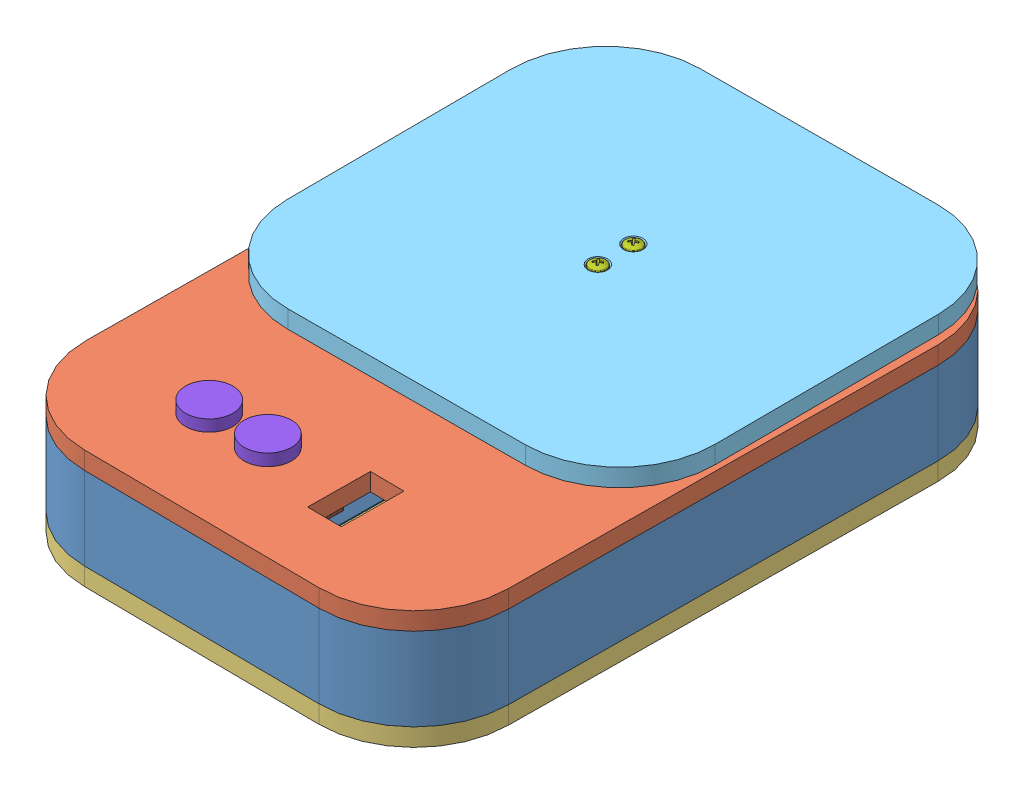
SolidWorks assembly Mainv1.1, configuration Default. Lengths in mm.
Overall size (189.66 80.65 261.56).
179 component instances, 44 part files, 6 mates.
Components (placement in the parent):
- Main-1: Main [Default] at (-331.7007 96.9527 454.1899) size (182.26 61.96 261.56)
  - mail wall-1: mail wall [Default] at (468.1099 74.0645 -181.95) x (-0.999962 0 -0.008727) z (0.008727 0 -0.999962) size (180 35 260)
  - top lid-1: top lid [Default] at (468.1099 116.5645 -181.95) x (-0.999962 0 -0.008727) z (0.008727 0 -0.999962) size (180 7.5 260)
  - bottom lid-2: bottom lid [Default] at (468.1099 31.5645 -181.95) x (0.999962 0 0.008727) z (-0.008727 0 0.999962) size (180 7.5 260)
  - Loadcell-1kg-No Name.step-1: Loadcell-1kg-No Name.step [Default] at (468.4825 94.8439 -197.5959) x (0 0 1) z (-1 0 0) size (91.8 14.23 13.91)
  - tray-1: tray [Default] at (468.6751 134.9439 -266.3463) x (0.999991 0 -0.00428) z (0.00428 0 0.999991) size (180 7.5 175)
  - Part5-1: Part5 [Default] at origin size (12.6 12.5 27.5)
  - pan cross head_am-1: pan cross head_am [B18.6.7M - M3.5 x 0.6 x 35 Type I Cross Recessed PHMS --35N] at (468.4825 128.4614 -232.8459) x (0 -1 0) z (-0.788636 0 0.61486) size (37.57 7 7)
  - pan cross head_am-3: pan cross head_am [B18.6.7M - M3.5 x 0.6 x 35 Type I Cross Recessed PHMS --35N] at (468.4825 128.5554 -217.8459) x (0 -1 0) z (0.792721 0 -0.609585) size (37.57 7 7)
  - Part1-1: Part1 [Default] at origin size (50 22.7 32.99)
  - hex bolt_am-1: hex bolt_am [B18.2.3.5M - Hex bolt M5 x 0.8 x 35 --16N] at (468.8184 72.2139 -162.6607) x (0 1 0) z (0 0 1) size (38.58 9.24 8)
  - hex bolt_am-2: hex bolt_am [B18.2.3.5M - Hex bolt M5 x 0.8 x 35 --16N] at (468.8184 72.2139 -177.7301) x (0 1 0) z (0 0 1) size (38.58 9.24 8)
- pcb_with_screws-1: pcb_with_screws [Default] at (347.1614 488.5879 -158.0964) x (0.371474 0 -0.928443) z (-0.928443 0 -0.371474) size (77.8 61.26 94.96)
  - pcb.step-1: pcb.step [Default] at (-541.6964 307.1593 96.7738) x (-0.93165 0 -0.363358) z (0 -1 0) size (48.01 79.98 16.61)
    - Board.step-1: Board.step [Default] at origin size (48.01 78.74 0.41)
      - Open CASCADE STEP translator 7.5 2.1.1.step-1: Open CASCADE STEP translator 7.5 2.1.1.step [Default] at (0 0 -0.4115) size (48.01 78.74 0.41)
    - HX711 out.step-1: HX711 out.step [Default] at origin size (10.16 2.54 10.59)
      - Header_4.step-1: Header_4.step [Default] at (27.685 46.598 -0.0051) x (0 -1 0) z (-1 0 0) size (2.54 10.59 10.16)
        - header.step-1: header.step [Default] at origin size (2.54 10.59 2.54)
          - header-0.step-1: header-0.step [Default] at origin size (2.54 8.5 2.54)
          - pin.step-1: pin.step [Default] at (-1.4 0 0) size (0.4 10 1.99)
        - header.step-2: header.step [Default] at (0 0 -2.54) size (2.54 10.59 2.54)
          - header-0.step-1: header-0.step [Default] at origin size (2.54 8.5 2.54)
          - pin.step-1: pin.step [Default] at (-1.4 0 0) size (0.4 10 1.99)
        - header.step-3: header.step [Default] at (0 0 -5.08) size (2.54 10.59 2.54)
          - header-0.step-1: header-0.step [Default] at origin size (2.54 8.5 2.54)
          - pin.step-1: pin.step [Default] at (-1.4 0 0) size (0.4 10 1.99)
        - header.step-4: header.step [Default] at (0 0 -7.62) size (2.54 10.59 2.54)
          - header-0.step-1: header-0.step [Default] at origin size (2.54 8.5 2.54)
          - pin.step-1: pin.step [Default] at (-1.4 0 0) size (0.4 10 1.99)
    - HX711_lc.step-1: HX711_lc.step [Default] at origin size (10.16 2.54 10.59)
      - Header_4.step-1: Header_4.step [Default] at (30.23 66.915 -0.0051) x (0 -1 0) z (-1 0 0) size (2.54 10.59 10.16)
        - header.step-1: header.step [Default] at origin size (2.54 10.59 2.54)
          - header-0.step-1: header-0.step [Default] at origin size (2.54 8.5 2.54)
          - pin.step-1: pin.step [Default] at (-1.4 0 0) size (0.4 10 1.99)
        - header.step-2: header.step [Default] at (0 0 -2.54) size (2.54 10.59 2.54)
          - header-0.step-1: header-0.step [Default] at origin size (2.54 8.5 2.54)
          - pin.step-1: pin.step [Default] at (-1.4 0 0) size (0.4 10 1.99)
        - header.step-3: header.step [Default] at (0 0 -5.08) size (2.54 10.59 2.54)
          - header-0.step-1: header-0.step [Default] at origin size (2.54 8.5 2.54)
          - pin.step-1: pin.step [Default] at (-1.4 0 0) size (0.4 10 1.99)
        - header.step-4: header.step [Default] at (0 0 -7.62) size (2.54 10.59 2.54)
          - header-0.step-1: header-0.step [Default] at origin size (2.54 8.5 2.54)
          - pin.step-1: pin.step [Default] at (-1.4 0 0) size (0.4 10 1.99)
    - usb 2.0.step-1: usb 2.0.step [Default] at origin size (7.8 5.5 3.71)
      - USB3090-30-A--3DModel-STEP-56544.step-1: USB3090-30-A--3DModel-STEP-56544.step [Default] at (7.762 1.514 0) x (1 0 0) z (0 -1 0) size (7.8 3.71 5.5)
    - R 470.step-1: R 470.step [Default] at origin size (2 1.25 0.6)
      - 6201218720.step-1: 6201218720.step [Default] at (15.687 7.62 0) x (1 0 0) z (0 0 1) size (2 1.25 0.6)
        - term1.step-1: term1.step [Default] at (-1 -0.625 0) size (0.35 1.25 0.6)
        - term2.step-1: term2.step [Default] at (0.65 -0.625 0) size (0.35 1.25 0.6)
        - body.step-1: body.step [Default] at (-0.65 -0.6125 0.006) size (1.3 1.22 0.59)
    - R 47k.step-1: R 47k.step [Default] at origin size (2 1.25 0.6)
      - 6062674512.step-1: 6062674512.step [Default] at (18.862 49.53 0) x (-1 0 0) z (0 0 1) size (2 1.25 0.6)
        - term1-1.step-1: term1-1.step [Default] at (-1 -0.625 0) size (0.35 1.25 0.6)
        - term2-2.step-1: term2-2.step [Default] at (0.65 -0.625 0) size (0.35 1.25 0.6)
        - body-3.step-1: body-3.step [Default] at (-0.65 -0.6125 0.006) size (1.3 1.22 0.59)
    - R 15k.step-1: R 15k.step [Default] at origin size (2 1.25 0.6)
      - 7267289360.step-1: 7267289360.step [Default] at (18.937 59.563 0) x (-1 0 0) z (0 0 1) size (2 1.25 0.6)
        - solidBody.step-1: solidBody.step [Default] at origin size (1.95 1.25 0.55)
        - Terminal.step-1: Terminal.step [Default] at origin size (2 1.25 0.6)
        - solidTop.step-1: solidTop.step [Default] at origin size (1.2 1.25 0.02)
    - R5-10K.step-1: R5-10K.step [Default] at origin size (1.6 0.8 0.55)
      - CRG0603F10K_10.step-1: CRG0603F10K_10.step [Default] at (45.212 17.526 0) x (1 0 0) z (0 -1 0) size (1.6 0.55 0.8)
    - R4-10K.step-1: R4-10K.step [Default] at origin size (1.6 0.8 0.55)
      - CRG0603F10K_10.step-1: CRG0603F10K_10.step [Default] at (45.212 22.7965 0) x (-1 0 0) z (0 1 0) size (1.6 0.55 0.8)
    - R3-10K.step-1: R3-10K.step [Default] at origin size (1.6 0.8 0.55)
      - CRG0603F10K_10.step-1: CRG0603F10K_10.step [Default] at (45.212 28.067 0) x (1 0 0) z (0 -1 0) size (1.6 0.55 0.8)
    - R 2k.step-1: R 2k.step [Default] at origin size (2 1.25 0.6)
      - 6062674512.step-1: 6062674512.step [Default] at (15.814 12.319 0) x (-1 0 0) z (0 0 1) size (2 1.25 0.6)
        - term1-1.step-1: term1-1.step [Default] at (-1 -0.625 0) size (0.35 1.25 0.6)
        - term2-2.step-1: term2-2.step [Default] at (0.65 -0.625 0) size (0.35 1.25 0.6)
        - body-3.step-1: body-3.step [Default] at (-0.65 -0.6125 0.006) size (1.3 1.22 0.59)
    - R2-10K.step-1: R2-10K.step [Default] at origin size (1.6 0.8 0.55)
      - CRG0603F10K_10.step-1: CRG0603F10K_10.step [Default] at (22.733 36.195 0) x (-1 0 0) z (0 1 0) size (1.6 0.55 0.8)
    - R1-10K.step-1: R1-10K.step [Default] at origin size (1.6 0.8 0.55)
      - CRG0603F10K_10.step-1: CRG0603F10K_10.step [Default] at (22.733 42.545 0) x (-1 0 0) z (0 1 0) size (1.6 0.55 0.8)
    - MCP73831.step-1: MCP73831.step [Default] at origin size (2.7 2.9 1.45)
      - MCP73831T-5ACI_OT.step-1: MCP73831T-5ACI_OT.step [Default] at (8.255 12.012 0) x (0 -1 0) z (-1 0 0) size (2.9 1.45 2.7)
    - LED.step-1: LED.step [Default] at origin size (3 1 2)
      - KPA-3010CGCK-Base.step-1: KPA-3010CGCK-Base.step [Default] at (16.51 1.651 0.508) x (-1 0 0) z (0 0 -1) size (2.16 1 1.02)
      - KPA-3010CGCK-Base-4.step-1: KPA-3010CGCK-Base-4.step [Default] at (16.51 1.651 0.508) x (-1 0 0) z (0 0 -1) size (3 1 1.22)
      - KPA-3010CGCK-Base-5.step-1: KPA-3010CGCK-Base-5.step [Default] at (16.51 1.651 0.508) x (-1 0 0) z (0 0 -1) size (0.9 1 0)
      - KPA-3010CGCK-Base-6.step-1: KPA-3010CGCK-Base-6.step [Default] at (16.51 1.651 0.508) x (-1 0 0) z (0 0 -1) size (0.8 1 0.02)
      - KPA-3010CGCK-Base-7.step-1: KPA-3010CGCK-Base-7.step [Default] at (16.51 1.651 0.508) x (-1 0 0) z (0 0 -1) size (2.96 1 0.96)
    - battery.step-1: battery.step [Default] at origin size (7.4 5.75 10.4)
      - 6062675712.step-1: 6062675712.step [Default] at (9.274 74.295 0) x (1 0 0) z (0 -1 0) size (7.4 10.4 5.75)
    - load cell.step-1: load cell.step [Default] at origin size (10.16 2.54 10.59)
      - Header_4.step-1: Header_4.step [Default] at (30.099 71.755 -0.0051) x (0 -1 0) z (-1 0 0) size (2.54 10.59 10.16)
        - header.step-1: header.step [Default] at origin size (2.54 10.59 2.54)
          - header-0.step-1: header-0.step [Default] at origin size (2.54 8.5 2.54)
          - pin.step-1: pin.step [Default] at (-1.4 0 0) size (0.4 10 1.99)
        - header.step-2: header.step [Default] at (0 0 -2.54) size (2.54 10.59 2.54)
          - header-0.step-1: header-0.step [Default] at origin size (2.54 8.5 2.54)
          - pin.step-1: pin.step [Default] at (-1.4 0 0) size (0.4 10 1.99)
        - header.step-3: header.step [Default] at (0 0 -5.08) size (2.54 10.59 2.54)
          - header-0.step-1: header-0.step [Default] at origin size (2.54 8.5 2.54)
          - pin.step-1: pin.step [Default] at (-1.4 0 0) size (0.4 10 1.99)
        - header.step-4: header.step [Default] at (0 0 -7.62) size (2.54 10.59 2.54)
          - header-0.step-1: header-0.step [Default] at origin size (2.54 8.5 2.54)
          - pin.step-1: pin.step [Default] at (-1.4 0 0) size (0.4 10 1.99)
    - buttons.step-1: buttons.step [Default] at origin size (2.54 10.16 10.59)
      - Header_4.step-1: Header_4.step [Default] at (39.497 59.817 -0.0051) x (-1 0 0) z (0 1 0) size (2.54 10.59 10.16)
        - header.step-1: header.step [Default] at origin size (2.54 10.59 2.54)
          - header-0.step-1: header-0.step [Default] at origin size (2.54 8.5 2.54)
          - pin.step-1: pin.step [Default] at (-1.4 0 0) size (0.4 10 1.99)
        - header.step-2: header.step [Default] at (0 0 -2.54) size (2.54 10.59 2.54)
          - header-0.step-1: header-0.step [Default] at origin size (2.54 8.5 2.54)
          - pin.step-1: pin.step [Default] at (-1.4 0 0) size (0.4 10 1.99)
        - header.step-3: header.step [Default] at (0 0 -5.08) size (2.54 10.59 2.54)
          - header-0.step-1: header-0.step [Default] at origin size (2.54 8.5 2.54)
          - pin.step-1: pin.step [Default] at (-1.4 0 0) size (0.4 10 1.99)
        - header.step-4: header.step [Default] at (0 0 -7.62) size (2.54 10.59 2.54)
          - header-0.step-1: header-0.step [Default] at origin size (2.54 8.5 2.54)
          - pin.step-1: pin.step [Default] at (-1.4 0 0) size (0.4 10 1.99)
    - OLED.step-1: OLED.step [Default] at origin size (2.54 10.16 16)
      - MTSW-104-22-S-S-420.step-1: MTSW-104-22-S-S-420.step [Default] at (44.831 57.277 0) x (0 -1 0) z (-1 0 0) size (10.16 16 2.54)
        - MTSW-104-22-S-420.step-1: MTSW-104-22-S-420.step [Default] at (0 -2.794 0) size (8.51 16 0.89)
        - MTSW-104-22-S-S-420_body.step-1: MTSW-104-22-S-S-420_body.step [Default] at origin size (10.16 2.54 2.54)
    - ESP-12F.step-1: ESP-12F.step [Default] at origin size (17.7 24.9 3.1)
      - ESP-12F-8.step-1: ESP-12F-8.step [Default] at (33.909 28.956 0) x (1 0 0) z (0 -1 0) size (17.7 3.1 24.9)
    - C5-4.7uF.step-1: C5-4.7uF.step [Default] at origin size (2 1.25 1.45)
      - 885012107013.step-1: 885012107013.step [Default] at (10.345 18.923 0) x (-1 0 0) z (0 0 1) size (2 1.25 1.45)
        - Fillet1.step-1: Fillet1.step [Default] at origin size (0.5 1.25 1.45)
        - Fillet2.step-1: Fillet2.step [Default] at origin size (0.5 1.25 1.45)
        - body2.step-1: body2.step [Default] at origin size (1 1.22 1.42)
    - C4-4.7uF.step-1: C4-4.7uF.step [Default] at origin size (2 1.25 1.45)
      - 885012107013.step-1: 885012107013.step [Default] at (11.245 26.543 0) x (1 0 0) z (0 0 1) size (2 1.25 1.45)
        - Fillet1.step-1: Fillet1.step [Default] at origin size (0.5 1.25 1.45)
        - Fillet2.step-1: Fillet2.step [Default] at origin size (0.5 1.25 1.45)
        - body2.step-1: body2.step [Default] at origin size (1 1.22 1.42)
    - C3-10uF.step-1: C3-10uF.step [Default] at origin size (5.3 4.5 5.5)
      - 865080340001.step-1: 865080340001.step [Default] at (10.737 64.643 0) x (-1 0 0) z (0 0 1) size (5.3 4.5 5.5)
        - Base.step-1: Base.step [Default] at origin size (4.5 4.5 1.6)
        - Pin1Fillet.step-1: Pin1Fillet.step [Default] at origin size (2.25 0.75 0.3)
        - Pin2Fillet.step-1: Pin2Fillet.step [Default] at origin size (2.25 0.75 0.3)
        - Fillet.step-1: Fillet.step [Default] at origin size (4.2 4.2 4.4)
      - 865080340001.step-2: 865080340001.step [Default] at (10.737 64.643 0) x (-1 0 0) z (0 0 1) size (5.3 4.5 5.5)
        - Base.step-1: Base.step [Default] at origin size (4.5 4.5 1.6)
        - Pin1Fillet.step-1: Pin1Fillet.step [Default] at origin size (2.25 0.75 0.3)
        - Pin2Fillet.step-1: Pin2Fillet.step [Default] at origin size (2.25 0.75 0.3)
        - Fillet.step-1: Fillet.step [Default] at origin size (4.2 4.2 4.4)
    - C2-10uF.step-1: C2-10uF.step [Default] at origin size (5.3 4.5 5.5)
      - 865080340001.step-1: 865080340001.step [Default] at (10.737 44.069 0) x (-1 0 0) z (0 0 1) size (5.3 4.5 5.5)
        - Base.step-1: Base.step [Default] at origin size (4.5 4.5 1.6)
        - Pin1Fillet.step-1: Pin1Fillet.step [Default] at origin size (2.25 0.75 0.3)
        - Pin2Fillet.step-1: Pin2Fillet.step [Default] at origin size (2.25 0.75 0.3)
        - Fillet.step-1: Fillet.step [Default] at origin size (4.2 4.2 4.4)
      - 865080340001.step-2: 865080340001.step [Default] at (10.737 44.069 0) x (-1 0 0) z (0 0 1) size (5.3 4.5 5.5)
        - Base.step-1: Base.step [Default] at origin size (4.5 4.5 1.6)
        - Pin1Fillet.step-1: Pin1Fillet.step [Default] at origin size (2.25 0.75 0.3)
        - Pin2Fillet.step-1: Pin2Fillet.step [Default] at origin size (2.25 0.75 0.3)
        - Fillet.step-1: Fillet.step [Default] at origin size (4.2 4.2 4.4)
    - C1-10uF.step-1: C1-10uF.step [Default] at origin size (5.3 4.5 5.5)
      - 865080340001.step-1: 865080340001.step [Default] at (33.583 11.303 0) x (-1 0 0) z (0 0 1) size (5.3 4.5 5.5)
        - Base.step-1: Base.step [Default] at origin size (4.5 4.5 1.6)
        - Pin1Fillet.step-1: Pin1Fillet.step [Default] at origin size (2.25 0.75 0.3)
        - Pin2Fillet.step-1: Pin2Fillet.step [Default] at origin size (2.25 0.75 0.3)
        - Fillet.step-1: Fillet.step [Default] at origin size (4.2 4.2 4.4)
      - 865080340001.step-2: 865080340001.step [Default] at (33.583 11.303 0) x (-1 0 0) z (0 0 1) size (5.3 4.5 5.5)
        - Base.step-1: Base.step [Default] at origin size (4.5 4.5 1.6)
        - Pin1Fillet.step-1: Pin1Fillet.step [Default] at origin size (2.25 0.75 0.3)
        - Pin2Fillet.step-1: Pin2Fillet.step [Default] at origin size (2.25 0.75 0.3)
        - Fillet.step-1: Fillet.step [Default] at origin size (4.2 4.2 4.4)
    - TC2117.step-1: TC2117.step [Default] at origin size (7.13 5.32 1.17)
      - TC2117-3.3VDBTR.step-1: TC2117-3.3VDBTR.step [Default] at (10.864 54.356 0) x (-1 0 0) z (0 0 1) size (7 5.32 1.17)
        - body.step-1: body.step [Default] at origin size (1.3 1.22 0.59)
        - PinsArrayL.step-1: PinsArrayL.step [Default] at origin size (1.75 5.32 1.17)
        - FilletPinR.step-1: FilletPinR.step [Default] at origin size (1.75 3 1.17)
      - TC2117-3.3VDBTR.step-2: TC2117-3.3VDBTR.step [Default] at (10.737 54.356 0) x (-1 0 0) z (0 0 1) size (7 5.32 1.17)
        - body.step-1: body.step [Default] at origin size (1.3 1.22 0.59)
        - PinsArrayL.step-1: PinsArrayL.step [Default] at origin size (1.75 5.32 1.17)
        - FilletPinR.step-1: FilletPinR.step [Default] at origin size (1.75 3 1.17)
  - Part36-1: Part36 [Default] at (-868.0076 716.489 235.6311) x (0.932186 0.214397 0.291656) z (-0.265595 0.952553 0.148668) size (53.08 79 35.65)
  - pan cross head_am-4: pan cross head_am [B18.6.7M - M2.5 x 0.45 x 5 Type I Cross Recessed PHMS --5N] at (-581.9119 305.0593 74.4096) x (0 1 0) z (-0.92188 0 0.387475) size (7.07 5 5)
  - pan cross head_am-5: pan cross head_am [B18.6.7M - M2.5 x 0.45 x 5 Type I Cross Recessed PHMS --5N] at (-556.4391 305.0593 9.0972) x (0 1 0) z (-0.72878 0 -0.684748) size (7.07 5 5)
  - pan cross head_am-6: pan cross head_am [B18.6.7M - M2.5 x 0.45 x 5 Type I Cross Recessed PHMS --5N] at (-515.9277 305.0593 24.761) x (0 1 0) z (0.615507 0 -0.788131) size (7.07 5 5)
  - pan cross head_am-7: pan cross head_am [B18.6.7M - M2.5 x 0.45 x 5 Type I Cross Recessed PHMS --5N] at (-541.4467 305.0593 90.1917) x (0 1 0) z (-0.986634 0 -0.162951) size (7.07 5 5)
- Part37^Mainv1.1-1: Part37^Mainv1.1 [Default] at (219.8491 208.2452 724.4221) x (-0.999992 0 -0.003909) z (0 1 0) size (19.97 19.97 5) (virtual)
- Part37^Mainv1.1-2: Part37^Mainv1.1 [Default] at (379.302 208.1045 610.0075) x (-0.834808 0 0.550541) z (0 1 0) size (19.97 19.97 5) (virtual)
Mates (geometry in assembly coordinates):
- Coincident1: coincident anti-aligned: plane of Main-1/bottom lid-2 through (85.6258 171.0172 361.8002) normal (0 1 0); circle of pcb_with_screws-1/Part36-1
- Coincident2: coincident anti-aligned: plane of Main-1/mail wall-1 through (55.3651 206.0172 391.5372) normal (0.999962 0 0.008727); plane of pcb_with_screws-1/pcb.step-1/Board.step-1/Open CASCADE STEP translator 7.5 2.1.1.step-1 through (56.0864 181.0172 308.8891) normal (-0.999962 0 -0.008727)
- Lock1: lock: unknown of Main-1/bottom lid-2; unknown of pcb_with_screws-1/Part36-1
- Concentric4: concentric anti-aligned: circle of Main-1/top lid-1; circle of Part37^Mainv1.1-2
- Concentric5: concentric anti-aligned: circle of Main-1/top lid-1; circle of Part37^Mainv1.1-1
- Concentric7: concentric aligned: cylinder of Main-1/bottom lid-2 through (222.0917 163.5172 272.9876) axis (0 -1 0) radius 1.7; cylinder of pan cross head_am-4 through (222.0917 109.9845 272.9876) axis (0 -1 0) radius 1.5
